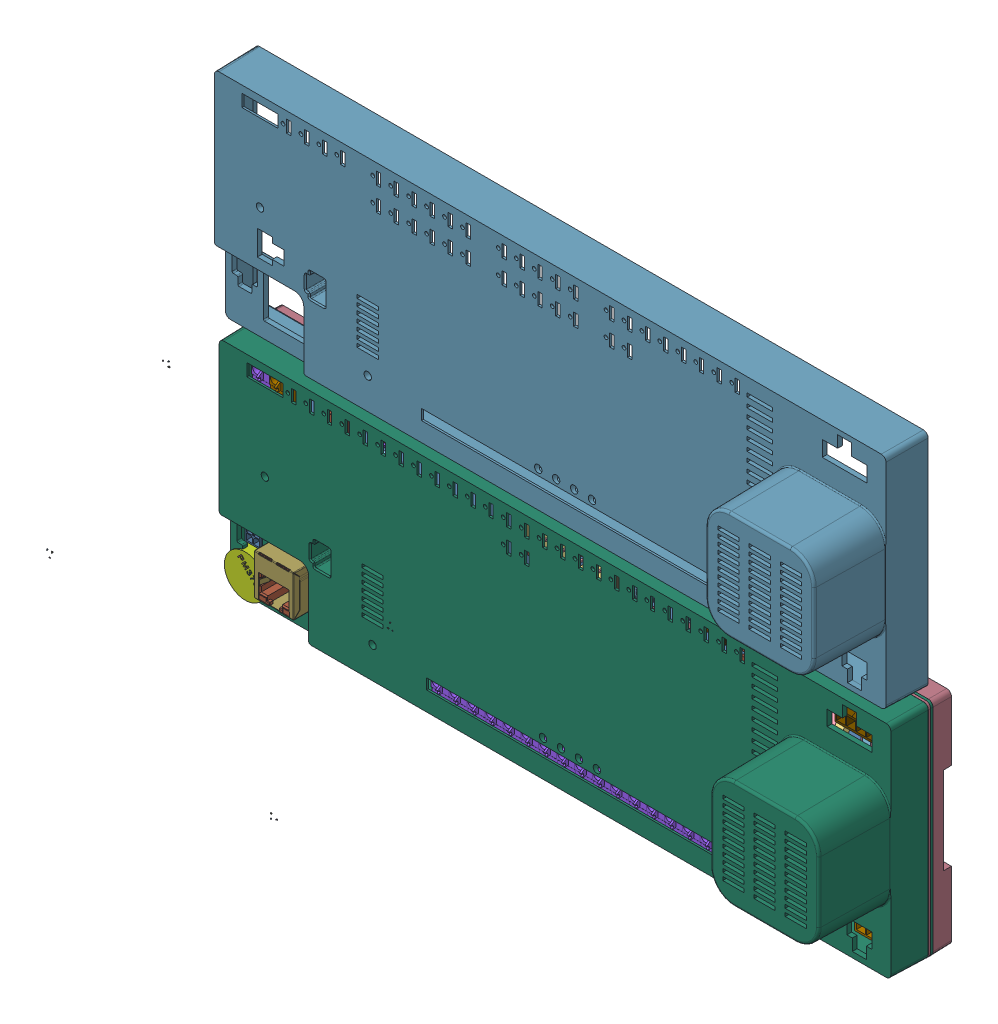
SolidWorks assembly _SC944D, configuration Default. Lengths in mm.
Overall size (351.19 158.64 58.89).
2950 component instances, 141 part files, 0 mates.
Components (placement in the parent):
- Board-1: Board [Default] at (0 0 -1.6703) size (281.94 89 1.67)
- D21-1: D21 [Default] at origin size (5.3 3.6 2.43)
  - SW3DPS-DIOD_SMD_10BF10-DEFAULT-1: SW3DPS-DIOD_SMD_10BF10-DEFAULT [Default] at (164.592 44.45 1.2) x (-1 0 0) z (0 1 0) size (5.3 2.43 3.6)
- J3-1: J3 [Default] at origin size (40.68 9.1 12.1)
  - STEP-61202621621-rev1-1: STEP-61202621621-rev1 [Default] at (135.8901 73.7931 4.4377) size (40.68 9.1 12.1)
    - 61202621621-1: 61202621621 [Default] at origin size (40.68 9.1 9.1)
    - 6120xx21621_PIN-1: 6120xx21621_PIN [Default] at (-15.24 1.27 -1.875) size (0.64 0.64 11.6)
    - 6120xx21621_PIN-2: 6120xx21621_PIN [Default] at (-15.24 -1.27 -1.875) size (0.64 0.64 11.6)
    - 6120xx21621_PIN-3: 6120xx21621_PIN [Default] at (-12.7 1.27 -1.875) size (0.64 0.64 11.6)
    - 6120xx21621_PIN-4: 6120xx21621_PIN [Default] at (-10.16 1.27 -1.875) size (0.64 0.64 11.6)
    - 6120xx21621_PIN-5: 6120xx21621_PIN [Default] at (-12.7 -1.27 -1.875) size (0.64 0.64 11.6)
    - 6120xx21621_PIN-6: 6120xx21621_PIN [Default] at (-10.16 -1.27 -1.875) size (0.64 0.64 11.6)
    - 6120xx21621_PIN-7: 6120xx21621_PIN [Default] at (-7.62 1.27 -1.875) size (0.64 0.64 11.6)
    - 6120xx21621_PIN-8: 6120xx21621_PIN [Default] at (-7.62 -1.27 -1.875) size (0.64 0.64 11.6)
    - 6120xx21621_PIN-9: 6120xx21621_PIN [Default] at (-5.08 1.27 -1.875) size (0.64 0.64 11.6)
    - 6120xx21621_PIN-10: 6120xx21621_PIN [Default] at (-5.08 -1.27 -1.875) size (0.64 0.64 11.6)
    - 6120xx21621_PIN-11: 6120xx21621_PIN [Default] at (-2.54 1.27 -1.875) size (0.64 0.64 11.6)
    - 6120xx21621_PIN-12: 6120xx21621_PIN [Default] at (0 1.27 -1.875) size (0.64 0.64 11.6)
    - 6120xx21621_PIN-13: 6120xx21621_PIN [Default] at (-2.54 -1.27 -1.875) size (0.64 0.64 11.6)
    - 6120xx21621_PIN-14: 6120xx21621_PIN [Default] at (0 -1.27 -1.875) size (0.64 0.64 11.6)
    - 6120xx21621_PIN-15: 6120xx21621_PIN [Default] at (2.54 1.27 -1.875) size (0.64 0.64 11.6)
    - 6120xx21621_PIN-16: 6120xx21621_PIN [Default] at (2.54 -1.27 -1.875) size (0.64 0.64 11.6)
    - 6120xx21621_PIN-17: 6120xx21621_PIN [Default] at (5.08 1.27 -1.875) size (0.64 0.64 11.6)
    - 6120xx21621_PIN-18: 6120xx21621_PIN [Default] at (7.62 1.27 -1.875) size (0.64 0.64 11.6)
    - 6120xx21621_PIN-19: 6120xx21621_PIN [Default] at (5.08 -1.27 -1.875) size (0.64 0.64 11.6)
    - 6120xx21621_PIN-20: 6120xx21621_PIN [Default] at (7.62 -1.27 -1.875) size (0.64 0.64 11.6)
    - 6120xx21621_PIN-21: 6120xx21621_PIN [Default] at (10.16 1.27 -1.875) size (0.64 0.64 11.6)
    - 6120xx21621_PIN-22: 6120xx21621_PIN [Default] at (12.7 1.27 -1.875) size (0.64 0.64 11.6)
    - 6120xx21621_PIN-23: 6120xx21621_PIN [Default] at (10.16 -1.27 -1.875) size (0.64 0.64 11.6)
    - 6120xx21621_PIN-24: 6120xx21621_PIN [Default] at (12.7 -1.27 -1.875) size (0.64 0.64 11.6)
    - 6120xx21621_PIN-25: 6120xx21621_PIN [Default] at (15.24 1.27 -1.875) size (0.64 0.64 11.6)
    - 6120xx21621_PIN-26: 6120xx21621_PIN [Default] at (15.24 -1.27 -1.875) size (0.64 0.64 11.6)
- R40-1: R40 [Default] at origin size (1.6 0.8 0.55)
  - RESC1608X84N-1: RESC1608X84N [Default] at (14.9226 63.5 0) x (1 0 0) z (0 -1 0) size (1.6 0.55 0.8)
- U28-1: U28 [Default] at origin size (8.2 5.4 2.15)
  - User_Library-SOIC-8-208-1: User_Library-SOIC-8-208 [Default] at (36.9887 35.7187 1.1652) x (0 1 0) z (1 0 0) size (5.4 2.15 8.2)
    - User_Library-SOIC-8-208_pin_SOIC_SOIC-208_1-1: User_Library-SOIC-8-208_pin_SOIC_SOIC-208_1 [Default] at (-1.905 0 2.7) size (0.4 1.25 1.4)
    - User_Library-SOIC-8-208_pin_SOIC_SOIC-208_1-2: User_Library-SOIC-8-208_pin_SOIC_SOIC-208_1 [Default] at (1.905 0 -2.7) x (-1 0 0) z (0 0 -1) size (0.4 1.25 1.4)
    - User_Library-SOIC-8-208_pin_SOIC_SOIC-208_1-3: User_Library-SOIC-8-208_pin_SOIC_SOIC-208_1 [Default] at (-0.635 0 2.7) size (0.4 1.25 1.4)
    - User_Library-SOIC-8-208_pin_SOIC_SOIC-208_1-4: User_Library-SOIC-8-208_pin_SOIC_SOIC-208_1 [Default] at (-1.905 0 -2.7) x (-1 0 0) z (0 0 -1) size (0.4 1.25 1.4)
    - User_Library-SOIC-8-208_pin_SOIC_SOIC-208_1-5: User_Library-SOIC-8-208_pin_SOIC_SOIC-208_1 [Default] at (0.635 0 2.7) size (0.4 1.25 1.4)
    - User_Library-SOIC-8-208_SOIC_150_SOIC_5.4x5.4_1-1: User_Library-SOIC-8-208_SOIC_150_SOIC_5.4x5.4_1 [Default] at origin size (5.4 2 5.4)
    - User_Library-SOIC-8-208_pin_SOIC_SOIC-208_1-6: User_Library-SOIC-8-208_pin_SOIC_SOIC-208_1 [Default] at (0.635 0 -2.7) x (-1 0 0) z (0 0 -1) size (0.4 1.25 1.4)
    - User_Library-SOIC-8-208_pin_SOIC_SOIC-208_1-7: User_Library-SOIC-8-208_pin_SOIC_SOIC-208_1 [Default] at (1.905 0 2.7) size (0.4 1.25 1.4)
    - User_Library-SOIC-8-208_pin_SOIC_SOIC-208_1-8: User_Library-SOIC-8-208_pin_SOIC_SOIC-208_1 [Default] at (-0.635 0 -2.7) x (-1 0 0) z (0 0 -1) size (0.4 1.25 1.4)
- C143-1: C143 [Default] at origin size (0.8 1.6 0.9)
  - User_Library-CAPC1608X09-1: User_Library-CAPC1608X09 [Default] at (40.9574 39.8463 0) x (0 1 0) z (0 0 1) size (1.6 0.8 0.9)
- C100-1: C100 [Default] at origin size (1.6 0.8 0.9)
  - User_Library-CAPC1608X09-1: User_Library-CAPC1608X09 [Default] at (55.5307 77.5652 0) x (-1 0 0) z (0 0 1) size (1.6 0.8 0.9)
- R171-1: R171 [Default] at origin size (0.8 1.6 0.55)
  - RESC1608X84N-1: RESC1608X84N [Default] at (24.9238 30.4799 0) x (0 -1 0) z (-1 0 0) size (1.6 0.55 0.8)
- R170-1: R170 [Default] at origin size (0.8 1.6 0.55)
  - RESC1608X84N-1: RESC1608X84N [Default] at (26.8287 30.4801 0) x (0 1 0) z (1 0 0) size (1.6 0.55 0.8)
- L42-1: L42 [Default] at origin size (1.6 0.8 0.9)
  - User_Library-CAPC1608X09-1: User_Library-CAPC1608X09 [Default] at (22.3838 31.1151 0) x (1 0 0) z (0 0 1) size (1.6 0.8 0.9)
- J53-1: J53 [Default] at origin size (6.9 9.6 16.3)
  - 64900211122-1: 64900211122 [Default] at (14.7469 31.4199 6.4152) x (0 -1 0) z (0 0 1) size (9.6 6.9 16.3)
    - 64900211122-1: 64900211122 [Default] at origin size (9.6 6.9 12.8)
    - 6490xx11122_PIN_1-1: 6490xx11122_PIN_1 [Default] at (-2.1 -0.025 -2.45) x (-1 0 0) z (0 0 -1) size (1.1 1.85 12.85)
    - 6490xx11122_PIN_1-2: 6490xx11122_PIN_1 [Default] at (2.1 -0.025 -2.45) x (-1 0 0) z (0 0 -1) size (1.1 1.85 12.85)
- D47-1: D47 [Default] at origin size (50.85 6.92 23.48)
  - SW3dPS-transistor_SOT233-1: SW3dPS-transistor_SOT233 [Default] at (-47.3774 4.0457 -21.9) x (-1 0 0) z (0 1 0) size (2.9 1.1 1.6)
  - SW3dPS-transistor_SOT233_1-1: SW3dPS-transistor_SOT233_1 [Default] at (-0.0474 0.004 -0.0219) x (-1 0 0) z (0 1 0) size (2.18 2.18 2.18)
  - SW3dPS-transistor_SOT233_2-1: SW3dPS-transistor_SOT233_2 [Default] at (0 0 0) x (-1 0 0) z (0 1 0) size (2.18 2.18 2.18)
  - SW3dPS-transistor_SOT233_3-1: SW3dPS-transistor_SOT233_3 [Default] x (-1 0 0) z (0 1 0) size (2.18 2.18 2.18)
- C138-1: C138 [Default] at origin size (0.8 1.6 0.9)
  - User_Library-CAPC1608X09-1: User_Library-CAPC1608X09 [Default] at (22.0663 27.1462 0) x (0 -1 0) z (0 0 1) size (1.6 0.8 0.9)
- R94-1: R94 [Default] at origin size (1.6 0.8 0.55)
  - RESC1608X84N-1: RESC1608X84N [Default] at (107.0609 46.9899 0) x (-1 0 0) z (0 1 0) size (1.6 0.55 0.8)
- R38-1: R38 [Default] at origin size (1.6 0.8 0.55)
  - RESC1608X84N-1: RESC1608X84N [Default] at (103.5049 27.8129 0) x (-1 0 0) z (0 1 0) size (1.6 0.55 0.8)
- D55-1: D55 [Default] at origin size (5.4 3.6 2.33)
  - SW3dPS-DO-214AA_SMB-1: SW3dPS-DO-214AA_SMB [Default] at (38.7092 48.4568 1.3) x (0 1 0) z (0 0 1) size (3.6 5.4 2.33)
- D44-1: D44 [Default] at origin size (7.95 5.9 2.33)
  - SW3dPS-DO-214AB_SMC-1: SW3dPS-DO-214AB_SMC [Default] at (38.71 48.4187 1.3) x (0 1 0) z (0 0 1) size (5.9 7.95 2.33)
- T20-1: T20 [Default] at origin size (6.73 10.1 2.41)
  - DPAK_TO-252AA_RGB8421504-1: DPAK_TO-252AA_RGB8421504 [Default] at (155.0668 27.3977 0.0428) x (-1 0 0) z (0 1 0) size (6.73 2.41 10.1)
- T19-1: T19 [Default] at origin size (6.73 10.1 2.41)
  - DPAK_TO-252AA_RGB8421504-1: DPAK_TO-252AA_RGB8421504 [Default] at (146.3038 27.3977 0.0428) x (-1 0 0) z (0 1 0) size (6.73 2.41 10.1)
- T17-1: T17 [Default] at origin size (6.73 10.1 2.41)
  - DPAK_TO-252AA_RGB8421504-1: DPAK_TO-252AA_RGB8421504 [Default] at (137.5408 27.3977 0.0428) x (-1 0 0) z (0 1 0) size (6.73 2.41 10.1)
- C16-1: C16 [Default] at origin size (1.6 0.8 0.9)
  - User_Library-CAPC1608X09-1: User_Library-CAPC1608X09 [Default] at (30.3212 53.3399 0) x (-1 0 0) z (0 0 1) size (1.6 0.8 0.9)
- R13-1: R13 [Default] at origin size (1.6 0.8 0.55)
  - RESC1608X84N-1: RESC1608X84N [Default] at (227.1712 72.8662 0) x (-1 0 0) z (0 1 0) size (1.6 0.55 0.8)
- D12-1: D12 [Default] at origin size (2.6 1.36 1.13)
  - SW3dPS-SOD-323-1: SW3dPS-SOD-323 [Default] at (215.9001 54.6101 0) x (1 0 0) z (0 0 1) size (2.6 1.36 1.13)
- L38-1: L38 [Default] at origin size (24.55 18 11.05)
  - WE-LF_SMD_SH-1: WE-LF_SMD_SH [Default] at (246.3987 5.6362 11.0652) x (1 0 0) z (0 0 1) size (24.55 18 11.05)
    - Pin-1: Pin [Default] at (9.325 -5 -11.05) size (2.95 5 6.45)
    - Pin-2: Pin [Default] at (9.325 5 -11.05) size (2.95 5 6.45)
    - Pin-3: Pin [Default] at (-9.325 -5 -11.05) x (-1 0 0) z (0 0 1) size (2.95 5 6.45)
    - Pin-4: Pin [Default] at (-9.325 5 -11.05) x (-1 0 0) z (0 0 1) size (2.95 5 6.45)
    - base_6-1: base_6 [Default] at origin size (18.65 4.43 7.08)
    - base_7-1: base_7 [Default] at origin size (13 13 5.01)
    - base_8-1: base_8 [Default] at origin size (23 18 10.6)
    - base_9-1: base_9 [Default] at origin size (18.65 4.43 7.08)
- L37-1: L37 [Default] at origin size (269.09 30.55 11.48)
  - User_Library-PM3700_1-1: User_Library-PM3700_1 [Default] at (246.3702 5.7247 0) x (0.707107 -0.707107 0) z (-0.707107 -0.707107 0) size (1.6 0.01 2.37)
  - User_Library-PM3700_2-1: User_Library-PM3700_2 [Default] at (0.2464 0.0057 0) x (0.707107 -0.707107 0) z (-0.707107 -0.707107 0) size (21.6 10.57 21.6)
  - User_Library-PM3700_3-1: User_Library-PM3700_3 [Default] at (0.0002 0 0) x (0.707107 -0.707107 0) z (-0.707107 -0.707107 0) size (0.5 10 0.64)
  - User_Library-PM3700_4-1: User_Library-PM3700_4 [Default] x (0.707107 -0.707107 0) z (-0.707107 -0.707107 0) size (1.6 0.01 2.38)
  - User_Library-PM3700_5-1: User_Library-PM3700_5 [Default] x (0.707107 -0.707107 0) z (-0.707107 -0.707107 0) size (1.6 0.01 2.35)
  - User_Library-PM3700_6-1: User_Library-PM3700_6 [Default] x (0.707107 -0.707107 0) z (-0.707107 -0.707107 0) size (14 6 14)
  - User_Library-PM3700_7-1: User_Library-PM3700_7 [Default] x (0.707107 -0.707107 0) z (-0.707107 -0.707107 0) size (2.22 0.01 2.32)
  - User_Library-PM3700_8-1: User_Library-PM3700_8 [Default] x (0.707107 -0.707107 0) z (-0.707107 -0.707107 0) size (1.81 0.01 2.32)
  - User_Library-PM3700_9-1: User_Library-PM3700_9 [Default] x (0.707107 -0.707107 0) z (-0.707107 -0.707107 0) size (1.55 0.01 2.25)
  - User_Library-PM3700_10-1: User_Library-PM3700_10 [Default] x (0.707107 -0.707107 0) z (-0.707107 -0.707107 0) size (4.21 10.45 7.86)
  - User_Library-PM3700_11-1: User_Library-PM3700_11 [Default] x (0.707107 -0.707107 0) z (-0.707107 -0.707107 0) size (7.86 10.45 4.21)
  - User_Library-PM3700_12-1: User_Library-PM3700_12 [Default] x (0.707107 -0.707107 0) z (-0.707107 -0.707107 0) size (4.21 10.45 7.86)
  - User_Library-PM3700-1: User_Library-PM3700 [Default] x (0.707107 -0.707107 0) z (-0.707107 -0.707107 0) size (7.86 10.45 4.21)
- C109-1: C109 [Default] at origin size (10.01 10 34.24)
  - CAP_ELE_10X31.5_E5.08MM-1: CAP_ELE_10X31.5_E5.08MM [Default] at (244.1574 49.5299 0) x (1 0 0) z (0 -1 0) size (10.01 32.74 10)
  - CAP_ELE_10X31.5_E5.08MM_2705478150-1: CAP_ELE_10X31.5_E5.08MM_2705478150 [Default] at (244.1574 49.5299 19) x (1 0 0) z (0 -1 0) size (10.01 15.24 10)
- R175-1: R175 [Default] at origin size (1.6 0.8 0.55)
  - RESC1608X84N-1: RESC1608X84N [Default] at (24.3841 44.196 0) x (1 0 0) z (0 -1 0) size (1.6 0.55 0.8)
- L17-1: L17 [Default] at origin size (0.8 1.6 0.9)
  - User_Library-CAPC1608X09-1: User_Library-CAPC1608X09 [Default] at (1.9049 48.1013 0) x (0 1 0) z (0 0 1) size (1.6 0.8 0.9)
- F5-1: F5 [Default] at origin size (14.4 22.52 14.67)
  - WE-SLM_744242-1: WE-SLM_744242 [Default] at (244.532 80.548 0) x (-1 0 0) z (0 -0.866025 0.5) size (14.4 3 20.8)
    - Extruded_11-1: Extruded_11 [Default] at origin size (14.4 3 20.8)
  - SW3dPS-PTCR,_240_V,_Raychem_LVR025S-1: SW3dPS-PTCR,_240_V,_Raychem_LVR025S [Default] at (247.042 78.359 0) x (-1 0 0) z (0 0.5 0.866026) size (8.66 19.48 3.6)
- D45-1: D45 [Default] at origin size (5.3 3.6 1.11)
  - 1175071672-1: 1175071672 [Default] at (226.5362 30.7975 0) size (5.3 3.6 1.1)
    - Extruded_12-1: Extruded_12 [Default] at origin size (5.3 3.6 1.1)
  - 1175071536-1: 1175071536 [Default] at (224.9996 30.7975 1.1) size (0.79 3.56 0.01)
    - Extruded_13-1: Extruded_13 [Default] at origin size (0.79 3.56 0.01)
- D40-1: D40 [Default] at origin size (5.3 3.6 1.11)
  - 1175071672-1: 1175071672 [Default] at (269.24 70.358 0) size (5.3 3.6 1.1)
    - Extruded_12-1: Extruded_12 [Default] at origin size (5.3 3.6 1.1)
  - 1175071536-1: 1175071536 [Default] at (267.7033 70.358 1.1) size (0.79 3.56 0.01)
    - Extruded_13-1: Extruded_13 [Default] at origin size (0.79 3.56 0.01)
- D39-1: D39 [Default] at origin size (5.3 3.6 1.11)
  - 1175071672-1: 1175071672 [Default] at (260.985 70.358 0) size (5.3 3.6 1.1)
    - Extruded_12-1: Extruded_12 [Default] at origin size (5.3 3.6 1.1)
  - 1175071536-1: 1175071536 [Default] at (262.5217 70.358 1.1) size (0.79 3.56 0.01)
    - Extruded_13-1: Extruded_13 [Default] at origin size (0.79 3.56 0.01)
- D29-1: D29 [Default] at origin size (3.6 5.3 1.11)
  - 1175071944-1: 1175071944 [Default] at (267.081 65.151 0) size (3.6 5.3 1.1)
    - Extruded_14-1: Extruded_14 [Default] at origin size (3.6 5.3 1.1)
  - 1175071808-1: 1175071808 [Default] at (267.081 63.6143 1.1) size (3.56 0.79 0.01)
    - Extruded_15-1: Extruded_15 [Default] at origin size (3.56 0.79 0.01)
- D28-1: D28 [Default] at origin size (3.6 5.3 1.11)
  - 1175071944-1: 1175071944 [Default] at (262.89 65.151 0) size (3.6 5.3 1.1)
    - Extruded_14-1: Extruded_14 [Default] at origin size (3.6 5.3 1.1)
  - 1175071808-1: 1175071808 [Default] at (262.89 63.6143 1.1) size (3.56 0.79 0.01)
    - Extruded_15-1: Extruded_15 [Default] at origin size (3.56 0.79 0.01)
- C1-1: C1 [Default] at origin size (1.6 0.8 0.9)
  - User_Library-CAPC1608X09-1: User_Library-CAPC1608X09 [Default] at (47.3076 70.9613 0) x (1 0 0) z (0 0 1) size (1.6 0.8 0.9)
- C2-1: C2 [Default] at origin size (1.6 0.8 0.9)
  - User_Library-CAPC1608X09-1: User_Library-CAPC1608X09 [Default] at (97.4091 75.1841 0) x (1 0 0) z (0 0 1) size (1.6 0.8 0.9)
- C3-1: C3 [Default] at origin size (1.6 0.8 0.9)
  - User_Library-CAPC1608X09-1: User_Library-CAPC1608X09 [Default] at (48.2601 66.6751 0) x (1 0 0) z (0 0 1) size (1.6 0.8 0.9)
- C4-1: C4 [Default] at origin size (0.8 1.6 0.9)
  - User_Library-CAPC1608X09-1: User_Library-CAPC1608X09 [Default] at (183.0388 49.2124 0) x (0 -1 0) z (0 0 1) size (1.6 0.8 0.9)
- C5-1: C5 [Default] at origin size (1.6 0.8 0.9)
  - User_Library-CAPC1608X09-1: User_Library-CAPC1608X09 [Default] at (131.8261 58.2931 0) x (1 0 0) z (0 0 1) size (1.6 0.8 0.9)
- C6-1: C6 [Default] at origin size (2 1.25 1)
  - User_Library-CAPC2013X10-1: User_Library-CAPC2013X10 [Default] at (73.7869 45.847 0) x (-1 0 0) z (0 0 1) size (2 1.25 1)
- C7-1: C7 [Default] at origin size (0.8 1.6 0.9)
  - User_Library-CAPC1608X09-1: User_Library-CAPC1608X09 [Default] at (116.5859 63.8811 0) x (0 1 0) z (0 0 1) size (1.6 0.8 0.9)
- C8-1: C8 [Default] at origin size (1.6 0.8 0.9)
  - User_Library-CAPC1608X09-1: User_Library-CAPC1608X09 [Default] at (27.1463 49.5301 0) x (1 0 0) z (0 0 1) size (1.6 0.8 0.9)
- C9-1: C9 [Default] at origin size (2 1.25 1)
  - User_Library-CAPC2013X10-1: User_Library-CAPC2013X10 [Default] at (162.9409 75.565 0) x (-1 0 0) z (0 0 1) size (2 1.25 1)
- C10-1: C10 [Default] at origin size (1.25 2 1)
  - User_Library-CAPC2013X10-1: User_Library-CAPC2013X10 [Default] at (185.674 68.0721 0) x (0 1 0) z (0 0 1) size (2 1.25 1)
- C11-1: C11 [Default] at origin size (2 1.25 1)
  - User_Library-CAPC2013X10-1: User_Library-CAPC2013X10 [Default] at (188.8489 68.834 0) x (-1 0 0) z (0 0 1) size (2 1.25 1)
- C13-1: C13 [Default] at origin size (18.01 18 56.04)
  - User_Library-Capacitor_Radial_Electrolitic-1: User_Library-Capacitor_Radial_Electrolitic [Default] at (265.3987 28.9199 1) x (1 0 0) z (0 -1 0) size (18.01 42.74 18)
  - 1173466560-1: 1173466560 [Default] at (261.6099 28.9199 -15) x (-1 0 0) z (0 0 1) size (0.8 0.8 15)
    - Cylinder_3-1: Cylinder_3 [Default] at origin size (0.8 0.8 15)
  - 1173466560-2: 1173466560 [Default] at (269.1099 28.92 -15) x (-1 0 0) z (0 0 1) size (0.8 0.8 15)
    - Cylinder_3-1: Cylinder_3 [Default] at origin size (0.8 0.8 15)
  - 1152710848-1: 1152710848 [Default] at (265.3987 28.9199 0) x (-1 0 0) z (0 0 1) size (12 12 1.5)
    - Cylinder_4-1: Cylinder_4 [Default] at origin size (12 12 1.5)
- C14-1: C14 [Default] at origin size (18.01 18 56.04)
  - User_Library-Capacitor_Radial_Electrolitic-1: User_Library-Capacitor_Radial_Electrolitic [Default] at (265.3987 49.9199 1) x (1 0 0) z (0 -1 0) size (18.01 42.74 18)
  - 1152710848-1: 1152710848 [Default] at (265.3987 49.9199 0) x (-1 0 0) z (0 0 1) size (12 12 1.5)
    - Cylinder_4-1: Cylinder_4 [Default] at origin size (12 12 1.5)
  - 1173466560-1: 1173466560 [Default] at (269.1099 49.92 -15) x (-1 0 0) z (0 0 1) size (0.8 0.8 15)
    - Cylinder_3-1: Cylinder_3 [Default] at origin size (0.8 0.8 15)
  - 1173466560-2: 1173466560 [Default] at (261.6099 49.9199 -15) x (-1 0 0) z (0 0 1) size (0.8 0.8 15)
    - Cylinder_3-1: Cylinder_3 [Default] at origin size (0.8 0.8 15)
- C15-1: C15 [Default] at origin size (18.01 18 56.04)
  - User_Library-Capacitor_Radial_Electrolitic-1: User_Library-Capacitor_Radial_Electrolitic [Default] at (244.3987 28.9199 1) x (1 0 0) z (0 -1 0) size (18.01 42.74 18)
  - 1173466560-1: 1173466560 [Default] at (240.6099 28.9199 -15) x (-1 0 0) z (0 0 1) size (0.8 0.8 15)
    - Cylinder_3-1: Cylinder_3 [Default] at origin size (0.8 0.8 15)
  - 1173466560-2: 1173466560 [Default] at (248.1099 28.92 -15) x (-1 0 0) z (0 0 1) size (0.8 0.8 15)
    - Cylinder_3-1: Cylinder_3 [Default] at origin size (0.8 0.8 15)
  - 1152710848-1: 1152710848 [Default] at (244.3987 28.9199 0) x (-1 0 0) z (0 0 1) size (12 12 1.5)
    - Cylinder_4-1: Cylinder_4 [Default] at origin size (12 12 1.5)
- C17-1: C17 [Default] at origin size (2.5 3.2 1.3)
  - User_Library-CAPC3225X13-1: User_Library-CAPC3225X13 [Default] at (256.7941 66.6749 0) x (0 -1 0) z (0 0 1) size (3.2 2.5 1.3)
- C18-1: C18 [Default] at origin size (0.8 1.6 0.9)
  - User_Library-CAPC1608X09-1: User_Library-CAPC1608X09 [Default] at (26.6064 63.5001 0) x (0 1 0) z (0 0 1) size (1.6 0.8 0.9)
- C19-1: C19 [Default] at origin size (3.2 2.5 1.3)
  - User_Library-CAPC3225X13-1: User_Library-CAPC3225X13 [Default] at (179.5462 45.2437 0) x (-1 0 0) z (0 0 1) size (3.2 2.5 1.3)
- C20-1: C20 [Default] at origin size (1.6 0.8 0.9)
  - User_Library-CAPC1608X09-1: User_Library-CAPC1608X09 [Default] at (39.8463 58.7376 0) x (1 0 0) z (0 0 1) size (1.6 0.8 0.9)
- C21-1: C21 [Default] at origin size (1.6 0.8 0.9)
  - User_Library-CAPC1608X09-1: User_Library-CAPC1608X09 [Default] at (27.9401 55.2451 0) size (1.6 0.8 0.9)
- C22-1: C22 [Default] at origin size (0.8 1.6 0.9)
  - User_Library-CAPC1608X09-1: User_Library-CAPC1608X09 [Default] at (28.0988 58.5787 0) x (0 -1 0) z (0 0 1) size (1.6 0.8 0.9)
- C23-1: C23 [Default] at origin size (2 1.25 1)
  - User_Library-CAPC2013X10-1: User_Library-CAPC2013X10 [Default] at (233.9976 69.5325 0) x (1 0 0) z (0 0 1) size (2 1.25 1)
- C24-1: C24 [Default] at origin size (1.6 0.8 0.9)
  - User_Library-CAPC1608X09-1: User_Library-CAPC1608X09 [Default] at (27.7812 47.6249 0) x (-1 0 0) z (0 0 1) size (1.6 0.8 0.9)
- C25-1: C25 [Default] at origin size (1.6 0.8 0.9)
  - User_Library-CAPC1608X09-1: User_Library-CAPC1608X09 [Default] at (68.5801 7.1438 0) x (1 0 0) z (0 0 1) size (1.6 0.8 0.9)
- C26-1: C26 [Default] at origin size (1.6 0.8 0.9)
  - User_Library-CAPC1608X09-1: User_Library-CAPC1608X09 [Default] at (65.7224 7.1437 0) x (-1 0 0) z (0 0 1) size (1.6 0.8 0.9)
- C27-1: C27 [Default] at origin size (1.6 0.8 0.9)
  - User_Library-CAPC1608X09-1: User_Library-CAPC1608X09 [Default] at (66.9926 40.6401 0) x (1 0 0) z (0 0 1) size (1.6 0.8 0.9)
- C28-1: C28 [Default] at origin size (1.6 0.8 0.9)
  - User_Library-CAPC1608X09-1: User_Library-CAPC1608X09 [Default] at (60.0074 40.3224 0) x (-1 0 0) z (0 0 1) size (1.6 0.8 0.9)
- C29-1: C29 [Default] at origin size (2 1.25 1)
  - User_Library-CAPC2013X10-1: User_Library-CAPC2013X10 [Default] at (164.5279 41.021 0) x (-1 0 0) z (0 0 1) size (2 1.25 1)
- C30-1: C30 [Default] at origin size (2 1.25 1)
  - User_Library-CAPC2013X10-1: User_Library-CAPC2013X10 [Default] at (164.5284 38.7985 0) x (-1 0 0) z (0 0 1) size (2 1.25 1)
- C31-1: C31 [Default] at origin size (0.8 1.6 0.9)
  - User_Library-CAPC1608X09-1: User_Library-CAPC1608X09 [Default] at (40.3226 43.3387 0) x (0 -1 0) z (0 0 1) size (1.6 0.8 0.9)
- C32-1: C32 [Default] at origin size (0.8 1.6 0.9)
  - User_Library-CAPC1608X09-1: User_Library-CAPC1608X09 [Default] at (71.5963 10.4139 0) x (0 -1 0) z (0 0 1) size (1.6 0.8 0.9)
- C33-1: C33 [Default] at origin size (0.8 1.6 0.9)
  - User_Library-CAPC1608X09-1: User_Library-CAPC1608X09 [Default] at (73.3426 10.4139 0) x (0 -1 0) z (0 0 1) size (1.6 0.8 0.9)
- C34-1: C34 [Default] at origin size (1.25 2 1)
  - User_Library-CAPC2013X10-1: User_Library-CAPC2013X10 [Default] at (43.6562 26.0351 0) x (0 1 0) z (0 0 1) size (2 1.25 1)
- C35-1: C35 [Default] at origin size (1.25 2 1)
  - User_Library-CAPC2013X10-1: User_Library-CAPC2013X10 [Default] at (74.93 27.3051 0) x (0 1 0) z (0 0 1) size (2 1.25 1)
- C36-1: C36 [Default] at origin size (0.8 1.6 0.9)
  - User_Library-CAPC1608X09-1: User_Library-CAPC1608X09 [Default] at (46.6726 21.1137 0) x (0 -1 0) z (0 0 1) size (1.6 0.8 0.9)
- C37-1: C37 [Default] at origin size (0.8 1.6 0.9)
  - User_Library-CAPC1608X09-1: User_Library-CAPC1608X09 [Default] at (66.1987 38.4176 0) x (0 1 0) z (0 0 1) size (1.6 0.8 0.9)
- C38-1: C38 [Default] at origin size (0.8 1.6 0.9)
  - User_Library-CAPC1608X09-1: User_Library-CAPC1608X09 [Default] at (60.9601 10.4139 0) x (0 -1 0) z (0 0 1) size (1.6 0.8 0.9)
- C39-1: C39 [Default] at origin size (0.8 1.6 0.9)
  - User_Library-CAPC1608X09-1: User_Library-CAPC1608X09 [Default] at (58.1659 38.1001 0) x (0 1 0) z (0 0 1) size (1.6 0.8 0.9)
- C40-1: C40 [Default] at origin size (0.8 1.6 0.9)
  - User_Library-CAPC1608X09-1: User_Library-CAPC1608X09 [Default] at (67.7862 38.4176 0) x (0 1 0) z (0 0 1) size (1.6 0.8 0.9)
- C41-1: C41 [Default] at origin size (0.8 1.6 0.9)
  - User_Library-CAPC1608X09-1: User_Library-CAPC1608X09 [Default] at (63.9763 10.4139 0) x (0 -1 0) z (0 0 1) size (1.6 0.8 0.9)
- C42-1: C42 [Default] at origin size (0.8 1.6 0.9)
  - User_Library-CAPC1608X09-1: User_Library-CAPC1608X09 [Default] at (73.1521 27.5589 0) x (0 -1 0) z (0 0 1) size (1.6 0.8 0.9)
- C43-1: C43 [Default] at origin size (1.6 0.8 0.9)
  - User_Library-CAPC1608X09-1: User_Library-CAPC1608X09 [Default] at (73.7871 18.4105 0) x (1 0 0) z (0 0 1) size (1.6 0.8 0.9)
- C44-1: C44 [Default] at origin size (1.6 0.8 0.9)
  - User_Library-CAPC1608X09-1: User_Library-CAPC1608X09 [Default] at (49.0219 11.3029 0) x (-1 0 0) z (0 0 1) size (1.6 0.8 0.9)
- C45-1: C45 [Default] at origin size (0.8 1.6 0.9)
  - User_Library-CAPC1608X09-1: User_Library-CAPC1608X09 [Default] at (46.5138 26.1937 0) x (0 -1 0) z (0 0 1) size (1.6 0.8 0.9)
- C46-1: C46 [Default] at origin size (0.8 1.6 0.9)
  - User_Library-CAPC1608X09-1: User_Library-CAPC1608X09 [Default] at (53.8162 37.9413 0) x (0 1 0) z (0 0 1) size (1.6 0.8 0.9)
- C47-1: C47 [Default] at origin size (2.5 3.2 1.3)
  - User_Library-CAPC3225X13-1: User_Library-CAPC3225X13 [Default] at (252.9841 66.6749 0) x (0 -1 0) z (0 0 1) size (3.2 2.5 1.3)
- C48-1: C48 [Default] at origin size (0.8 1.6 0.9)
  - User_Library-CAPC1608X09-1: User_Library-CAPC1608X09 [Default] at (250.3487 66.1988 0) x (0 1 0) z (0 0 1) size (1.6 0.8 0.9)
- C49-1: C49 [Default] at origin size (2 1.25 1)
  - User_Library-CAPC2013X10-1: User_Library-CAPC2013X10 [Default] at (153.7971 64.262 0) x (1 0 0) z (0 0 1) size (2 1.25 1)
- C50-1: C50 [Default] at origin size (1.6 0.8 0.9)
  - User_Library-CAPC1608X09-1: User_Library-CAPC1608X09 [Default] at (247.8088 73.0251 0) x (1 0 0) z (0 0 1) size (1.6 0.8 0.9)
- C51-1: C51 [Default] at origin size (3.2 1.6 1)
  - User_Library-CAPC3216X10-1: User_Library-CAPC3216X10 [Default] at (230.6638 51.7526 0) x (1 0 0) z (0 0 1) size (3.2 1.6 1)
- C52-1: C52 [Default] at origin size (3.2 1.6 1)
  - User_Library-CAPC3216X10-1: User_Library-CAPC3216X10 [Default] at (231.9337 35.0837 0) x (-1 0 0) z (0 0 1) size (3.2 1.6 1)
- C53-1: C53 [Default] at origin size (0.8 1.6 0.9)
  - User_Library-CAPC1608X09-1: User_Library-CAPC1608X09 [Default] at (225.9013 68.4212 0) x (0 -1 0) z (0 0 1) size (1.6 0.8 0.9)
- C54-1: C54 [Default] at origin size (1.25 2 1)
  - User_Library-CAPC2013X10-1: User_Library-CAPC2013X10 [Default] at (22.86 23.3679 0) x (0 -1 0) z (0 0 1) size (2 1.25 1)
- C55-1: C55 [Default] at origin size (0.8 1.6 0.9)
  - User_Library-CAPC1608X09-1: User_Library-CAPC1608X09 [Default] at (73.1519 23.7491 0) x (0 1 0) z (0 0 1) size (1.6 0.8 0.9)
- C56-1: C56 [Default] at origin size (1.6 0.8 0.9)
  - User_Library-CAPC1608X09-1: User_Library-CAPC1608X09 [Default] at (49.0219 13.8429 0) x (-1 0 0) z (0 0 1) size (1.6 0.8 0.9)
- C57-1: C57 [Default] at origin size (0.8 1.6 0.9)
  - User_Library-CAPC1608X09-1: User_Library-CAPC1608X09 [Default] at (53.9751 10.0012 0) x (0 -1 0) z (0 0 1) size (1.6 0.8 0.9)
- C58-1: C58 [Default] at origin size (2 1.25 1)
  - User_Library-CAPC2013X10-1: User_Library-CAPC2013X10 [Default] at (17.7801 19.304 0) x (1 0 0) z (0 0 1) size (2 1.25 1)
- C59-1: C59 [Default] at origin size (1.6 0.8 0.9)
  - User_Library-CAPC1608X09-1: User_Library-CAPC1608X09 [Default] at (173.7359 75.6919 0) x (-1 0 0) z (0 0 1) size (1.6 0.8 0.9)
- C60-1: C60 [Default] at origin size (1.6 0.8 0.9)
  - User_Library-CAPC1608X09-1: User_Library-CAPC1608X09 [Default] at (59.3724 49.2124 0) x (-1 0 0) z (0 0 1) size (1.6 0.8 0.9)
- C61-1: C61 [Default] at origin size (1.6 0.8 0.9)
  - User_Library-CAPC1608X09-1: User_Library-CAPC1608X09 [Default] at (29.7179 12.0649 0) x (-1 0 0) z (0 0 1) size (1.6 0.8 0.9)
- C62-1: C62 [Default] at origin size (1.6 0.8 0.9)
  - User_Library-CAPC1608X09-1: User_Library-CAPC1608X09 [Default] at (42.2276 17.6213 0) x (1 0 0) z (0 0 1) size (1.6 0.8 0.9)
- C63-1: C63 [Default] at origin size (1.6 3.2 1)
  - User_Library-CAPC3216X10-1: User_Library-CAPC3216X10 [Default] at (26.0351 20.6692 0) x (0 -1 0) z (0 0 1) size (3.2 1.6 1)
- C64-1: C64 [Default] at origin size (1.6 0.8 0.9)
  - User_Library-CAPC1608X09-1: User_Library-CAPC1608X09 [Default] at (39.5287 5.2387 0) x (-1 0 0) z (0 0 1) size (1.6 0.8 0.9)
- C65-1: C65 [Default] at origin size (1.6 0.8 0.9)
  - User_Library-CAPC1608X09-1: User_Library-CAPC1608X09 [Default] at (42.8624 5.2387 0) x (-1 0 0) z (0 0 1) size (1.6 0.8 0.9)
- C66-1: C66 [Default] at origin size (2 1.25 1)
  - User_Library-CAPC2013X10-1: User_Library-CAPC2013X10 [Default] at (247.8086 68.7387 0) x (-1 0 0) z (0 0 1) size (2 1.25 1)
- C67-1: C67 [Default] at origin size (1.6 0.8 0.9)
  - User_Library-CAPC1608X09-1: User_Library-CAPC1608X09 [Default] at (36.3537 5.2387 0) x (-1 0 0) z (0 0 1) size (1.6 0.8 0.9)
- C68-1: C68 [Default] at origin size (1.6 0.8 0.9)
  - User_Library-CAPC1608X09-1: User_Library-CAPC1608X09 [Default] at (21.1138 20.6376 0) x (1 0 0) z (0 0 1) size (1.6 0.8 0.9)
- C69-1: C69 [Default] at origin size (1.6 0.8 0.9)
  - User_Library-CAPC1608X09-1: User_Library-CAPC1608X09 [Default] at (21.1138 19.0501 0) x (1 0 0) z (0 0 1) size (1.6 0.8 0.9)
- C70-1: C70 [Default] at origin size (1.6 3.2 1)
  - User_Library-CAPC3216X10-1: User_Library-CAPC3216X10 [Default] at (23.9712 59.5313 0) x (0 1 0) z (0 0 1) size (3.2 1.6 1)
- C71-1: C71 [Default] at origin size (1.6 0.8 0.9)
  - User_Library-CAPC1608X09-1: User_Library-CAPC1608X09 [Default] at (16.6369 22.6059 0) x (-1 0 0) z (0 0 1) size (1.6 0.8 0.9)
- C72-1: C72 [Default] at origin size (1.6 0.8 0.9)
  - User_Library-CAPC1608X09-1: User_Library-CAPC1608X09 [Default] at (16.6369 21.0819 0) x (-1 0 0) z (0 0 1) size (1.6 0.8 0.9)
- C77-1: C77 [Default] at origin size (0.8 1.6 0.9)
  - User_Library-CAPC1608X09-1: User_Library-CAPC1608X09 [Default] at (228.2826 68.4212 0) x (0 -1 0) z (0 0 1) size (1.6 0.8 0.9)
- C79-1: C79 [Default] at origin size (1.6 0.8 0.9)
  - User_Library-CAPC1608X09-1: User_Library-CAPC1608X09 [Default] at (4.0995 19.4309 0) x (-1 0 0) z (0 0 1) size (1.6 0.8 0.9)
- C80-1: C80 [Default] at origin size (1.6 0.8 0.9)
  - User_Library-CAPC1608X09-1: User_Library-CAPC1608X09 [Default] at (6.9495 19.4311 0) x (1 0 0) z (0 0 1) size (1.6 0.8 0.9)
- C83-1: C83 [Default] at origin size (1.6 3.2 1)
  - User_Library-CAPC3216X10-1: User_Library-CAPC3216X10 [Default] at (26.1937 59.5313 0) x (0 1 0) z (0 0 1) size (3.2 1.6 1)
- C84-1: C84 [Default] at origin size (1.6 0.8 0.9)
  - User_Library-CAPC1608X09-1: User_Library-CAPC1608X09 [Default] at (181.9269 53.4669 0) x (-1 0 0) z (0 0 1) size (1.6 0.8 0.9)
- C85-1: C85 [Default] at origin size (1.6 0.8 0.9)
  - User_Library-CAPC1608X09-1: User_Library-CAPC1608X09 [Default] at (73.4061 50.9271 0) x (1 0 0) z (0 0 1) size (1.6 0.8 0.9)
- C86-1: C86 [Default] at origin size (0.8 1.6 0.9)
  - User_Library-CAPC1608X09-1: User_Library-CAPC1608X09 [Default] at (10.3188 21.1137 0) x (0 -1 0) z (0 0 1) size (1.6 0.8 0.9)
- C87-1: C87 [Default] at origin size (0.8 1.6 0.9)
  - User_Library-CAPC1608X09-1: User_Library-CAPC1608X09 [Default] at (0.0001 22.3519 0) x (0 -1 0) z (0 0 1) size (1.6 0.8 0.9)
- C88-1: C88 [Default] at origin size (2 1.25 1)
  - User_Library-CAPC2013X10-1: User_Library-CAPC2013X10 [Default] at (7.3026 53.34 0) x (1 0 0) z (0 0 1) size (2 1.25 1)
- C89-1: C89 [Default] at origin size (1.6 0.8 0.9)
  - User_Library-CAPC1608X09-1: User_Library-CAPC1608X09 [Default] at (14.9224 65.0874 0) x (-1 0 0) z (0 0 1) size (1.6 0.8 0.9)
- C90-1: C90 [Default] at origin size (2.5 3.2 1.3)
  - User_Library-CAPC3225X13-1: User_Library-CAPC3225X13 [Default] at (9.6838 29.4899 0) x (0 -1 0) z (0 0 1) size (3.2 2.5 1.3)
- C91-1: C91 [Default] at origin size (2 1.25 1)
  - User_Library-CAPC2013X10-1: User_Library-CAPC2013X10 [Default] at (3.6511 53.34 0) x (-1 0 0) z (0 0 1) size (2 1.25 1)
- C92-1: C92 [Default] at origin size (0.8 1.6 0.9)
  - User_Library-CAPC1608X09-1: User_Library-CAPC1608X09 [Default] at (10.9537 54.1338 0) x (0 1 0) z (0 0 1) size (1.6 0.8 0.9)
- C93-1: C93 [Default] at origin size (1.6 0.8 0.9)
  - User_Library-CAPC1608X09-1: User_Library-CAPC1608X09 [Default] at (9.0488 64.1351 0) x (1 0 0) z (0 0 1) size (1.6 0.8 0.9)
- C94-1: C94 [Default] at origin size (0.8 1.6 0.9)
  - User_Library-CAPC1608X09-1: User_Library-CAPC1608X09 [Default] at (199.6439 68.0721 0) x (0 1 0) z (0 0 1) size (1.6 0.8 0.9)
- C95-1: C95 [Default] at origin size (2 1.25 1)
  - User_Library-CAPC2013X10-1: User_Library-CAPC2013X10 [Default] at (247.8086 70.9612 0) x (-1 0 0) z (0 0 1) size (2 1.25 1)
- C96-1: C96 [Default] at origin size (0.8 1.6 0.9)
  - User_Library-CAPC1608X09-1: User_Library-CAPC1608X09 [Default] at (34.1312 41.1163 0) x (0 1 0) z (0 0 1) size (1.6 0.8 0.9)
- C97-1: C97 [Default] at origin size (0.8 1.6 0.9)
  - User_Library-CAPC1608X09-1: User_Library-CAPC1608X09 [Default] at (193.3574 59.0551 0) x (0 1 0) z (0 0 1) size (1.6 0.8 0.9)
- C98-1: C98 [Default] at origin size (1.25 2 1)
  - User_Library-CAPC2013X10-1: User_Library-CAPC2013X10 [Default] at (191.4525 59.3724 0) x (0 -1 0) z (0 0 1) size (2 1.25 1)
- C99-1: C99 [Default] at origin size (5.46 17.78 12)
  - 1175072352-1: 1175072352 [Default] at (221.8372 5.08 0) size (5.46 17.78 12)
    - Extruded_16-1: Extruded_16 [Default] at origin size (5.46 17.78 12)
- C101-1: C101 [Default] at origin size (2 1.25 1)
  - User_Library-CAPC2013X10-1: User_Library-CAPC2013X10 [Default] at (181.9271 55.245 0) x (1 0 0) z (0 0 1) size (2 1.25 1)
- C102-1: C102 [Default] at origin size (0.8 1.6 0.9)
  - User_Library-CAPC1608X09-1: User_Library-CAPC1608X09 [Default] at (69.8499 10.4141 0) x (0 1 0) z (0 0 1) size (1.6 0.8 0.9)
- C103-1: C103 [Default] at origin size (0.8 1.6 0.9)
  - User_Library-CAPC1608X09-1: User_Library-CAPC1608X09 [Default] at (65.7861 56.0425 0) x (0 -1 0) z (0 0 1) size (1.6 0.8 0.9)
- C104-1: C104 [Default] at origin size (1.6 0.8 0.9)
  - User_Library-CAPC1608X09-1: User_Library-CAPC1608X09 [Default] at (73.5331 48.1331 0) x (1 0 0) z (0 0 1) size (1.6 0.8 0.9)
- C105-1: C105 [Default] at origin size (2 1.25 1)
  - User_Library-CAPC2013X10-1: User_Library-CAPC2013X10 [Default] at (78.6131 48.8951 0) x (1 0 0) z (0 0 1) size (2 1.25 1)
- C106-1: C106 [Default] at origin size (0.8 1.6 0.9)
  - User_Library-CAPC1608X09-1: User_Library-CAPC1608X09 [Default] at (81.4071 35.0519 0) x (0 -1 0) z (0 0 1) size (1.6 0.8 0.9)
- C107-1: C107 [Default] at origin size (1.6 0.8 0.9)
  - User_Library-CAPC1608X09-1: User_Library-CAPC1608X09 [Default] at (74.0409 43.6879 0) x (-1 0 0) z (0 0 1) size (1.6 0.8 0.9)
- C108-1: C108 [Default] at origin size (2 1.25 1)
  - User_Library-CAPC2013X10-1: User_Library-CAPC2013X10 [Default] at (78.7399 33.02 0) x (-1 0 0) z (0 0 1) size (2 1.25 1)
- C110-1: C110 [Default] at origin size (3.2 1.6 1)
  - User_Library-CAPC3216X10-1: User_Library-CAPC3216X10 [Default] at (71.9137 57.1499 0) x (-1 0 0) z (0 0 1) size (3.2 1.6 1)
- C111-1: C111 [Default] at origin size (1.6 0.8 0.9)
  - User_Library-CAPC1608X09-1: User_Library-CAPC1608X09 [Default] at (78.7399 46.7359 0) x (-1 0 0) z (0 0 1) size (1.6 0.8 0.9)
- C112-1: C112 [Default] at origin size (0.8 1.6 0.9)
  - User_Library-CAPC1608X09-1: User_Library-CAPC1608X09 [Default] at (181.1338 49.2124 0) x (0 -1 0) z (0 0 1) size (1.6 0.8 0.9)
- C113-1: C113 [Default] at origin size (0.8 1.6 0.9)
  - User_Library-CAPC1608X09-1: User_Library-CAPC1608X09 [Default] at (-3.1749 43.1799 0) x (0 -1 0) z (0 0 1) size (1.6 0.8 0.9)
- C114-1: C114 [Default] at origin size (1.6 0.8 0.9)
  - User_Library-CAPC1608X09-1: User_Library-CAPC1608X09 [Default] at (2.2226 25.5588 0) x (1 0 0) z (0 0 1) size (1.6 0.8 0.9)
- C115-1: C115 [Default] at origin size (0.8 1.6 0.9)
  - User_Library-CAPC1608X09-1: User_Library-CAPC1608X09 [Default] at (-3.1751 28.8926 0) x (0 1 0) z (0 0 1) size (1.6 0.8 0.9)
- C117-1: C117 [Default] at origin size (0.8 1.6 0.9)
  - User_Library-CAPC1608X09-1: User_Library-CAPC1608X09 [Default] at (-3.1749 39.3699 0) x (0 -1 0) z (0 0 1) size (1.6 0.8 0.9)
- C118-1: C118 [Default] at origin size (3.2 1.6 1)
  - User_Library-CAPC3216X10-1: User_Library-CAPC3216X10 [Default] at (224.1549 51.7524 0) x (-1 0 0) z (0 0 1) size (3.2 1.6 1)
- C119-1: C119 [Default] at origin size (1.6 0.8 0.9)
  - User_Library-CAPC1608X09-1: User_Library-CAPC1608X09 [Default] at (67.7619 53.3399 0) x (-1 0 0) z (0 0 1) size (1.6 0.8 0.9)
- D1-1: D1 [Default] at origin size (35.65 149.6 23.48)
  - SW3dPS-transistor_SOT233-1: SW3dPS-transistor_SOT233 [Default] at (32.7794 146.12 -21.9) x (0 1 0) z (1 0 0) size (2.9 1.1 1.6)
  - SW3dPS-transistor_SOT233_1-1: SW3dPS-transistor_SOT233_1 [Default] at (0.0328 0.1461 -0.0219) x (0 1 0) z (1 0 0) size (2.18 2.18 2.18)
  - SW3dPS-transistor_SOT233_2-1: SW3dPS-transistor_SOT233_2 [Default] at (0 0.0001 0) x (0 1 0) z (1 0 0) size (2.18 2.18 2.18)
  - SW3dPS-transistor_SOT233_3-1: SW3dPS-transistor_SOT233_3 [Default] x (0 1 0) z (1 0 0) size (2.18 2.18 2.18)
- D2-1: D2 [Default] at origin size (31.49 48.03 23.48)
  - SW3dPS-transistor_SOT233-1: SW3dPS-transistor_SOT233 [Default] at (-28.0099 45.1619 -21.9) x (-1 0 0) z (0 1 0) size (2.9 1.1 1.6)
  - SW3dPS-transistor_SOT233_1-1: SW3dPS-transistor_SOT233_1 [Default] at (-0.028 0.0452 -0.0219) x (-1 0 0) z (0 1 0) size (2.18 2.18 2.18)
  - SW3dPS-transistor_SOT233_2-1: SW3dPS-transistor_SOT233_2 [Default] at (0 0 0) x (-1 0 0) z (0 1 0) size (2.18 2.18 2.18)
  - SW3dPS-transistor_SOT233_3-1: SW3dPS-transistor_SOT233_3 [Default] x (-1 0 0) z (0 1 0) size (2.18 2.18 2.18)
- D3-1: D3 [Default] at origin size (169.38 102.14 23.48)
  - SW3dPS-transistor_SOT233-1: SW3dPS-transistor_SOT233 [Default] at (165.9002 99.2688 -21.9) x (1 0 0) z (0 -1 0) size (2.9 1.1 1.6)
  - SW3dPS-transistor_SOT233_1-1: SW3dPS-transistor_SOT233_1 [Default] at (0.1659 0.0993 -0.0219) x (1 0 0) z (0 -1 0) size (2.18 2.18 2.18)
  - SW3dPS-transistor_SOT233_2-1: SW3dPS-transistor_SOT233_2 [Default] at (0.0002 0.0001 0) x (1 0 0) z (0 -1 0) size (2.18 2.18 2.18)
  - SW3dPS-transistor_SOT233_3-1: SW3dPS-transistor_SOT233_3 [Default] x (1 0 0) z (0 -1 0) size (2.18 2.18 2.18)
- D4-1: D4 [Default] at origin size (46.47 40.25 23.48)
  - SW3dPS-transistor_SOT233-1: SW3dPS-transistor_SOT233 [Default] at (43.0148 37.3832 -21.9) x (-1 0 0) z (0 1 0) size (2.9 1.1 1.6)
  - SW3dPS-transistor_SOT233_1-1: SW3dPS-transistor_SOT233_1 [Default] at (0.043 0.0374 -0.0219) x (-1 0 0) z (0 1 0) size (2.18 2.18 2.18)
  - SW3dPS-transistor_SOT233_2-1: SW3dPS-transistor_SOT233_2 [Default] at (0 0 0) x (-1 0 0) z (0 1 0) size (2.18 2.18 2.18)
  - SW3dPS-transistor_SOT233_3-1: SW3dPS-transistor_SOT233_3 [Default] x (-1 0 0) z (0 1 0) size (2.18 2.18 2.18)
- D5-1: D5 [Default] at origin size (102.39 23.96 23.48)
  - SW3dPS-transistor_SOT233-1: SW3dPS-transistor_SOT233 [Default] at (99.5228 -20.4852 -21.9) x (0 -1 0) z (-1 0 0) size (2.9 1.1 1.6)
  - SW3dPS-transistor_SOT233_1-1: SW3dPS-transistor_SOT233_1 [Default] at (0.0995 -0.0205 -0.0219) x (0 -1 0) z (-1 0 0) size (2.18 2.18 2.18)
  - SW3dPS-transistor_SOT233_2-1: SW3dPS-transistor_SOT233_2 [Default] at (0.0001 0 0) x (0 -1 0) z (-1 0 0) size (2.18 2.18 2.18)
  - SW3dPS-transistor_SOT233_3-1: SW3dPS-transistor_SOT233_3 [Default] x (0 -1 0) z (-1 0 0) size (2.18 2.18 2.18)
- D6-1: D6 [Default] at origin size (1.36 2.6 1.13)
  - SW3dPS-SOD-323-1: SW3dPS-SOD-323 [Default] at (130.9371 61.3053 0) x (0 -1 0) z (0 0 1) size (2.6 1.36 1.13)
- D7-1: D7 [Default] at origin size (1.36 2.6 1.13)
  - SW3dPS-SOD-323-1: SW3dPS-SOD-323 [Default] at (128.9051 61.2698 0) x (0 -1 0) z (0 0 1) size (2.6 1.36 1.13)
- D8-1: D8 [Default] at origin size (2.6 5.2 2.43)
  - SW3dPS-DO-214AC_SMA-1: SW3dPS-DO-214AC_SMA [Default] at (37.0205 68.453 1.3) x (1 0 0) z (0 0 1) size (2.6 5.2 2.43)
- D9-1: D9 [Default] at origin size (2.6 5.2 2.43)
  - SW3dPS-DO-214AC_SMA-1: SW3dPS-DO-214AC_SMA [Default] at (52.705 68.8975 1.3) x (1 0 0) z (0 0 1) size (2.6 5.2 2.43)
- D10-1: D10 [Default] at origin size (5.2 2.6 2.43)
  - SW3dPS-DO-214AC_SMA-1: SW3dPS-DO-214AC_SMA [Default] at (152.527 67.183 1.3) x (0 -1 0) z (0 0 1) size (2.6 5.2 2.43)
- D11-1: D11 [Default] at origin size (136.36 83.28 23.48)
  - SW3dPS-transistor_SOT233-1: SW3dPS-transistor_SOT233 [Default] at (132.8802 80.4093 -21.9) x (1 0 0) z (0 -1 0) size (2.9 1.1 1.6)
  - SW3dPS-transistor_SOT233_1-1: SW3dPS-transistor_SOT233_1 [Default] at (0.1329 0.0804 -0.0219) x (1 0 0) z (0 -1 0) size (2.18 2.18 2.18)
  - SW3dPS-transistor_SOT233_2-1: SW3dPS-transistor_SOT233_2 [Default] at (0.0001 0.0001 0) x (1 0 0) z (0 -1 0) size (2.18 2.18 2.18)
  - SW3dPS-transistor_SOT233_3-1: SW3dPS-transistor_SOT233_3 [Default] x (1 0 0) z (0 -1 0) size (2.18 2.18 2.18)
